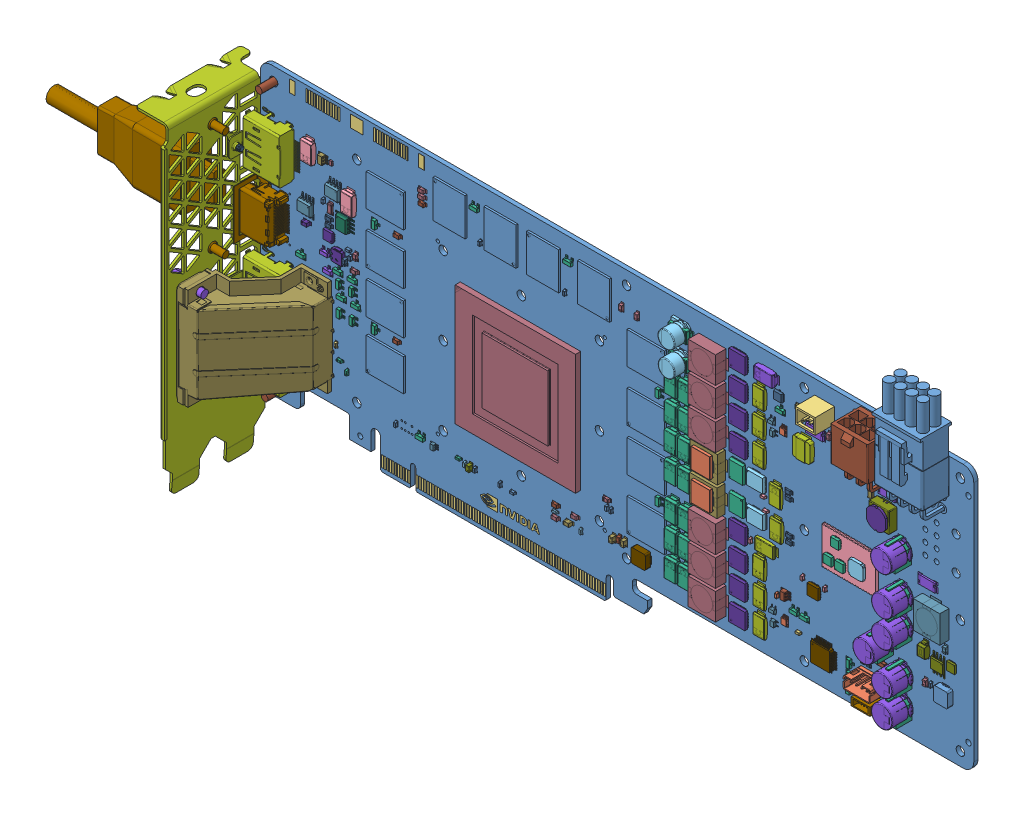
SolidWorks assembly PG600 SKU 0 3D Model, configuration Default. Lengths in mm.
Overall size (340.29 147.26 41.89).
548 component instances, 102 part files, 0 mates.
Components (placement in the parent):
- 142-1G600-1000-A05-1: 142-1G600-1000-A05 [Default] at origin size (266.7 111.15 1.57)
- 085-0009-000_1-1: 085-0009-000_1 [Default] at (20.943 18.972 0) x (1 0 0) z (0 0 -1) size (4.7 8 1.1)
- 075-0186-000_1-1: 075-0186-000_1 [Default] at (174.857 94.825 1.575) x (-1 0 0) z (0 0 1) size (7.4 5.75 10.67)
- 092-0023-000_1-1: 092-0023-000_1 [Default] at (-32.5 68.3 1.575) x (-1 0 0) z (0 0 1) size (3.05 1.35 0.81)
- 041-0139-000_1-1: 041-0139-000_1 [Default] at (120.487 94.534 1.575) x (-1 0 0) z (0 0 1) size (8.76 6.6 6.13)
- 041-0139-000_1-2: 041-0139-000_1 [Default] at (120.582 85.179 1.575) x (-1 0 0) z (0 0 1) size (8.76 6.6 6.13)
- CAP_SMD_066X066_B_6000_GREY-1: CAP_SMD_066X066_B_6000_GREY [Default] at (195.893 32.152 1.575) x (0 -1 0) z (0 0 1) size (8.76 6.8 6)
- CAP_SMD_066X066_B_6000_GREY-2: CAP_SMD_066X066_B_6000_GREY [Default] at (202.884 24.662 1.575) x (0 -1 0) z (0 0 1) size (8.76 6.8 6)
- CAP_SMD_066X066_B_6000_GREY-3: CAP_SMD_066X066_B_6000_GREY [Default] at (202.882 14.586 1.575) x (0 -1 0) z (0 0 1) size (8.76 6.8 6)
- CAP_SMD_066X066_B_6000_GREY-4: CAP_SMD_066X066_B_6000_GREY [Default] at (202.893 40.377 1.575) x (0 -1 0) z (0 0 1) size (8.76 6.8 6)
- CAP_SMD_066X066_B_6000_GREY-5: CAP_SMD_066X066_B_6000_GREY [Default] at (202.941 50.414 1.575) x (0 -1 0) z (0 0 1) size (8.76 6.8 6)
- CAP_SMD_066X066_B_6000_GREY-6: CAP_SMD_066X066_B_6000_GREY [Default] at (202.578 64.708 1.575) x (0 -1 0) z (0 0 1) size (8.76 6.8 6)
- 080-1128-000_3-1: 080-1128-000_3 [Default] at (-34.025 79.504 1.575) size (15.59 18.32 13.18)
- 080-1128-000_3-2: 080-1128-000_3 [Default] at (-34.025 11.683 1.575) size (15.59 18.32 13.18)
- 080-1128-000_3-3: 080-1128-000_3 [Default] at (-34.025 34.29 1.575) size (15.59 18.32 13.18)
- 032-0286-000_1-1: 032-0286-000_1 [Default] at (195.95 32.23 1.575) x (0 1 0) z (0 0 1) size (8 8 10.56)
- 032-0286-000_1-2: 032-0286-000_1 [Default] at (202.578 64.708 1.575) x (0 1 0) z (0 0 1) size (8 8 10.56)
- 032-0286-000_1-3: 032-0286-000_1 [Default] at (202.884 24.662 1.575) x (0 1 0) z (0 0 1) size (8 8 10.56)
- 032-0286-000_1-4: 032-0286-000_1 [Default] at (202.882 14.586 1.575) x (0 1 0) z (0 0 1) size (8 8 10.56)
- 032-0286-000_1-5: 032-0286-000_1 [Default] at (202.893 40.377 1.575) x (0 1 0) z (0 0 1) size (8 8 10.56)
- 032-0286-000_1-6: 032-0286-000_1 [Default] at (202.941 50.414 1.575) x (0 1 0) z (0 0 1) size (8 8 10.56)
- 065-0573-000_3-1: 065-0573-000_3 [Default] at (191.77 10.711 1.575) size (7.8 4.2 4.7)
- 195-2659-000_1-1: 195-2659-000_1 [Default] at (-11.4 64.9 1.575) x (-1 0 0) z (0 0 1) size (3.05 1.27 0.65)
- 195-2659-000_1-2: 195-2659-000_1 [Default] at (-11.4 62.7 1.575) x (-1 0 0) z (0 0 1) size (3.05 1.27 0.65)
- 039-0122-000_1-1: 039-0122-000_1 [Default] at (35.525 33.7 0) x (1 0 0) z (0 0 -1) size (3.05 1.27 0.95)
- 039-0122-000_1-2: 039-0122-000_1 [Default] at (72.9 71.075 0) x (0 -1 0) z (0 0 -1) size (3.05 1.27 0.95)
- 039-0127-000_1-1: 039-0127-000_1 [Default] at (55.7 37.85 0) x (1 0 0) z (0 0 -1) size (3.05 1.27 1.5)
- 039-0123-000_1-1: 039-0123-000_1 [Default] at (-2.83 51.24 0) x (0 -1 0) z (0 0 -1) size (3.05 1.27 0.95)
- 039-0123-000_1-2: 039-0123-000_1 [Default] at (10.45 18.82 0) x (1 0 0) z (0 0 -1) size (3.05 1.27 0.95)
- 039-0123-000_1-3: 039-0123-000_1 [Default] at (-0.72 49.54 0) x (0 -1 0) z (0 0 -1) size (3.05 1.27 0.95)
- 039-0123-000_1-4: 039-0123-000_1 [Default] at (-1.775 55.408 0) x (0 -1 0) z (0 0 -1) size (3.05 1.27 0.95)
- 039-0123-000_1-5: 039-0123-000_1 [Default] at (-1.76 64.49 0) x (0 -1 0) z (0 0 -1) size (3.05 1.27 0.95)
- 039-0123-000_1-6: 039-0123-000_1 [Default] at (-1.9 76.4 0) x (0 -1 0) z (0 0 -1) size (3.05 1.27 0.95)
- 039-0123-000_1-7: 039-0123-000_1 [Default] at (-2 83.1 0) x (0 -1 0) z (0 0 -1) size (3.05 1.27 0.95)
- 039-0123-000_1-8: 039-0123-000_1 [Default] at (22.11 26.9 0) x (1 0 0) z (0 0 -1) size (3.05 1.27 0.95)
- 195-2659-000_1-3: 195-2659-000_1 [Default] at (188.38 21.821 1.575) x (0 -1 0) z (0 0 1) size (3.05 1.27 0.65)
- 195-2659-000_1-4: 195-2659-000_1 [Default] at (190.5 21.844 1.575) x (0 -1 0) z (0 0 1) size (3.05 1.27 0.65)
- 039-0122-000_1-3: 039-0122-000_1 [Default] at (-20.619 61.841 0) x (1 0 0) z (0 0 -1) size (3.05 1.27 0.95)
- 039-0183-000_1-1: 039-0183-000_1 [Default] at (172.15 38.75 0) x (0 1 0) z (0 0 -1) size (3.05 1.27 0.95)
- 039-0123-000_1-9: 039-0123-000_1 [Default] at (-10.025 67.525 0) x (-1 0 0) z (0 0 -1) size (3.05 1.27 0.95)
- 039-0123-000_1-10: 039-0123-000_1 [Default] at (175.7 88 1.575) x (0 1 0) z (0 0 1) size (3.05 1.27 0.95)
- 039-0123-000_1-11: 039-0123-000_1 [Default] at (180.3 85.6 1.575) x (-1 0 0) z (0 0 1) size (3.05 1.27 0.95)
- 039-0123-000_1-12: 039-0123-000_1 [Default] at (184.3 88.7 1.575) x (0 -1 0) z (0 0 1) size (3.05 1.27 0.95)
- 195-1593-000_1-1: 195-1593-000_1 [Default] at (162.725 84.45 0) x (1 0 0) z (0 0 -1) size (3.05 1.27 0.7)
- 195-1593-000_1-2: 195-1593-000_1 [Default] at (162.75 82.3 0) x (1 0 0) z (0 0 -1) size (3.05 1.27 0.7)
- 039-0123-000_1-13: 039-0123-000_1 [Default] at (6.35 17.11 0) x (-1 0 0) z (0 0 -1) size (3.05 1.27 0.95)
- 039-0123-000_1-14: 039-0123-000_1 [Default] at (-1.3 57.63 1.575) x (0 -1 0) z (0 0 1) size (3.05 1.27 0.95)
- 039-0123-000_1-15: 039-0123-000_1 [Default] at (-1.855 72.5 0) x (0 -1 0) z (0 0 -1) size (3.05 1.27 0.95)
- 039-0123-000_1-16: 039-0123-000_1 [Default] at (-1.725 52.725 1.575) size (3.05 1.27 0.95)
- 039-0123-000_1-17: 039-0123-000_1 [Default] at (83.95 31.45 0) x (0 1 0) z (0 0 -1) size (3.05 1.27 0.95)
- 039-0123-000_1-18: 039-0123-000_1 [Default] at (80.65 14.5 1.575) x (-1 0 0) z (0 0 1) size (3.05 1.27 0.95)
- 039-0123-000_1-19: 039-0123-000_1 [Default] at (73.405 10.52 1.575) x (-1 0 0) z (0 0 1) size (3.05 1.27 0.95)
- 039-0123-000_1-20: 039-0123-000_1 [Default] at (86.1 31.8 0) x (0 1 0) z (0 0 -1) size (3.05 1.27 0.95)
- 039-0123-000_1-21: 039-0123-000_1 [Default] at (211.708 26.314 1.575) x (0 1 0) z (0 0 1) size (3.05 1.27 0.95)
- 039-0149-000_1-1: 039-0149-000_1 [Default] at (41.5 10.9 1.575) x (0 -1 0) z (0 0 1) size (3.05 1.27 1.45)
- 039-0122-000_1-4: 039-0122-000_1 [Default] at (96.025 17.979 0) x (0 1 0) z (0 0 -1) size (3.05 1.27 0.95)
- 039-0122-000_1-5: 039-0122-000_1 [Default] at (73.428 14.643 1.575) x (-1 0 0) z (0 0 1) size (3.05 1.27 0.95)
- 039-0123-000_1-22: 039-0123-000_1 [Default] at (35.525 42.275 0) x (1 0 0) z (0 0 -1) size (3.05 1.27 0.95)
- 039-0123-000_1-23: 039-0123-000_1 [Default] at (49.833 47.9 0) x (1 0 0) z (0 0 -1) size (3.05 1.27 0.95)
- 039-0122-000_1-6: 039-0122-000_1 [Default] at (35.525 59.075 0) x (1 0 0) z (0 0 -1) size (3.05 1.27 0.95)
- 039-0127-000_1-2: 039-0127-000_1 [Default] at (78.45 11.45 1.575) x (-1 0 0) z (0 0 1) size (3.05 1.27 1.5)
- 039-0122-000_1-7: 039-0122-000_1 [Default] at (97.194 15.396 1.575) x (0 -1 0) z (0 0 1) size (3.05 1.27 0.95)
- 039-0123-000_1-24: 039-0123-000_1 [Default] at (98.646 15.219 0) x (-1 0 0) z (0 0 -1) size (3.05 1.27 0.95)
- 039-0123-000_1-25: 039-0123-000_1 [Default] at (69.8 34.95 0) x (0 1 0) z (0 0 -1) size (3.05 1.27 0.95)
- 039-0123-000_1-26: 039-0123-000_1 [Default] at (92.545 26 1.575) size (3.05 1.27 0.95)
- 039-0123-000_1-27: 039-0123-000_1 [Default] at (103.581 14.199 0) x (0 -1 0) z (0 0 -1) size (3.05 1.27 0.95)
- 039-0127-000_1-3: 039-0127-000_1 [Default] at (95.03 14.63 1.575) x (0 -1 0) z (0 0 1) size (3.05 1.27 1.5)
- 039-0127-000_1-4: 039-0127-000_1 [Default] at (99.35 15.506 1.575) x (0 -1 0) z (0 0 1) size (3.05 1.27 1.5)
- 039-0123-000_1-28: 039-0123-000_1 [Default] at (95.803 14.546 0) x (0 1 0) z (0 0 -1) size (3.05 1.27 0.95)
- 039-0127-000_1-5: 039-0127-000_1 [Default] at (52.698 38.9 0) x (0 -1 0) z (0 0 -1) size (3.05 1.27 1.5)
- 039-0127-000_1-6: 039-0127-000_1 [Default] at (67.63 38.9 0) x (0 -1 0) z (0 0 -1) size (3.05 1.27 1.5)
- 039-0127-000_1-7: 039-0127-000_1 [Default] at (55.7 39.955 0) x (-1 0 0) z (0 0 -1) size (3.05 1.27 1.5)
- 039-0127-000_1-8: 039-0127-000_1 [Default] at (64.677 39.955 0) x (1 0 0) z (0 0 -1) size (3.05 1.27 1.5)
- 039-0127-000_1-9: 039-0127-000_1 [Default] at (64.673 37.85 0) x (-1 0 0) z (0 0 -1) size (3.05 1.27 1.5)
- 039-0127-000_1-10: 039-0127-000_1 [Default] at (59.55 50.825 0) x (1 0 0) z (0 0 -1) size (3.05 1.27 1.5)
- 039-0127-000_1-11: 039-0127-000_1 [Default] at (59.55 52.95 0) x (-1 0 0) z (0 0 -1) size (3.05 1.27 1.5)
- 039-0127-000_1-12: 039-0127-000_1 [Default] at (58.745 55.905 0) x (0 -1 0) z (0 0 -1) size (3.05 1.27 1.5)
- 039-0127-000_1-13: 039-0127-000_1 [Default] at (70.425 47.9 0) x (-1 0 0) z (0 0 -1) size (3.05 1.27 1.5)
- 039-0127-000_1-14: 039-0127-000_1 [Default] at (70.425 54 0) x (-1 0 0) z (0 0 -1) size (3.05 1.27 1.5)
- 039-0123-000_1-29: 039-0123-000_1 [Default] at (84.925 50.525 0) x (-1 0 0) z (0 0 -1) size (3.05 1.27 0.95)
- 039-0123-000_1-30: 039-0123-000_1 [Default] at (47.5 71.075 0) x (0 -1 0) z (0 0 -1) size (3.05 1.27 0.95)
- 039-0123-000_1-31: 039-0123-000_1 [Default] at (61.695 56.125 0) x (0 -1 0) z (0 0 -1) size (3.05 1.27 0.95)
- 039-0123-000_1-32: 039-0123-000_1 [Default] at (84.2 34.825 0) x (0 -1 0) z (0 0 -1) size (3.05 1.27 0.95)
- 039-0123-000_1-33: 039-0123-000_1 [Default] at (-25.756 82.681 0) x (-1 0 0) z (0 0 -1) size (3.05 1.27 0.95)
- 039-0183-000_1-2: 039-0183-000_1 [Default] at (219.175 40.665 1.575) x (0 1 0) z (0 0 1) size (3.05 1.27 0.95)
- 195-2659-000_1-5: 195-2659-000_1 [Default] at (156.375 93.375 0) x (-1 0 0) z (0 0 -1) size (3.05 1.27 0.65)
- 039-0123-000_1-34: 039-0123-000_1 [Default] at (113.785 14.62 0) x (0 1 0) z (0 0 -1) size (3.05 1.27 0.95)
- 039-0123-000_1-35: 039-0123-000_1 [Default] at (24.275 48.025 0) x (-1 0 0) z (0 0 -1) size (3.05 1.27 0.95)
- 039-0123-000_1-36: 039-0123-000_1 [Default] at (24.225 45.55 0) x (-1 0 0) z (0 0 -1) size (3.05 1.27 0.95)
- 039-0123-000_1-37: 039-0123-000_1 [Default] at (118.603 81.12 0) x (0 1 0) z (0 0 -1) size (3.05 1.27 0.95)
- 039-0123-000_1-38: 039-0123-000_1 [Default] at (118.603 73.283 0) x (0 1 0) z (0 0 -1) size (3.05 1.27 0.95)
- 039-0123-000_1-39: 039-0123-000_1 [Default] at (118.603 66.408 0) x (0 1 0) z (0 0 -1) size (3.05 1.27 0.95)
- 039-0123-000_1-40: 039-0123-000_1 [Default] at (120.142 63.5 0) x (-1 0 0) z (0 0 -1) size (3.05 1.27 0.95)
- 039-0123-000_1-41: 039-0123-000_1 [Default] at (118.7 49.1 0) x (0 -1 0) z (0 0 -1) size (3.05 1.27 0.95)
- 039-0123-000_1-42: 039-0123-000_1 [Default] at (118.603 38.283 0) x (0 1 0) z (0 0 -1) size (3.05 1.27 0.95)
- 039-0123-000_1-43: 039-0123-000_1 [Default] at (118.603 31.408 0) x (0 1 0) z (0 0 -1) size (3.05 1.27 0.95)
- 039-0123-000_1-44: 039-0123-000_1 [Default] at (118.603 21.008 0) x (0 -1 0) z (0 0 -1) size (3.05 1.27 0.95)
- 039-0123-000_1-45: 039-0123-000_1 [Default] at (114 89.35 0) x (1 0 0) z (0 0 -1) size (3.05 1.27 0.95)
- 039-0123-000_1-46: 039-0123-000_1 [Default] at (103.9 90.95 0) x (0 -1 0) z (0 0 -1) size (3.05 1.27 0.95)
- 039-0123-000_1-47: 039-0123-000_1 [Default] at (103.9 90.95 1.575) x (0 -1 0) z (0 0 1) size (3.05 1.27 0.95)
- 039-0123-000_1-48: 039-0123-000_1 [Default] at (98.101 90.925 1.575) x (0 -1 0) z (0 0 1) size (3.05 1.27 0.95)
- 039-0122-000_1-8: 039-0122-000_1 [Default] at (14 37.95 1.575) x (-1 0 0) z (0 0 1) size (3.05 1.27 0.95)
- 039-0123-000_1-49: 039-0123-000_1 [Default] at (23.428 91.558 1.575) x (-1 0 0) z (0 0 1) size (3.05 1.27 0.95)
- 039-0123-000_1-50: 039-0123-000_1 [Default] at (23.5 89.1 0) x (-1 0 0) z (0 0 -1) size (3.05 1.27 0.95)
- 039-0122-000_1-9: 039-0122-000_1 [Default] at (23.546 87.229 1.575) x (-1 0 0) z (0 0 1) size (3.05 1.27 0.95)
- 039-0123-000_1-51: 039-0123-000_1 [Default] at (23.428 89.433 1.575) x (-1 0 0) z (0 0 1) size (3.05 1.27 0.95)
- 039-0123-000_1-52: 039-0123-000_1 [Default] at (21.8 85.9 0) x (1 0 0) z (0 0 -1) size (3.05 1.27 0.95)
- 039-0122-000_1-10: 039-0122-000_1 [Default] at (14.275 72.275 1.575) x (-1 0 0) z (0 0 1) size (3.05 1.27 0.95)
- 039-0183-000_1-3: 039-0183-000_1 [Default] at (150.05 23.325 1.575) x (0 1 0) z (0 0 1) size (3.05 1.27 0.95)
- 039-0183-000_1-4: 039-0183-000_1 [Default] at (150 32.875 1.575) x (0 1 0) z (0 0 1) size (3.05 1.27 0.95)
- 039-0183-000_1-5: 039-0183-000_1 [Default] at (148.667 70.869 0) x (-1 0 0) z (0 0 -1) size (3.05 1.27 0.95)
- 039-0183-000_1-6: 039-0183-000_1 [Default] at (148.66 87.864 0) x (0 1 0) z (0 0 -1) size (3.05 1.27 0.95)
- 039-0183-000_1-7: 039-0183-000_1 [Default] at (149.052 17.91 0) x (0 -1 0) z (0 0 -1) size (3.05 1.27 0.95)
- 039-0183-000_1-8: 039-0183-000_1 [Default] at (157.626 48.088 1.575) x (0 1 0) z (0 0 1) size (3.05 1.27 0.95)
- 039-0183-000_1-9: 039-0183-000_1 [Default] at (155.25 48.082 1.575) x (0 1 0) z (0 0 1) size (3.05 1.27 0.95)
- 039-0183-000_1-10: 039-0183-000_1 [Default] at (154.836 59.015 1.575) x (0 -1 0) z (0 0 1) size (3.05 1.27 0.95)
- 039-0183-000_1-11: 039-0183-000_1 [Default] at (157.186 59.015 1.575) x (0 -1 0) z (0 0 1) size (3.05 1.27 0.95)
- 039-0183-000_1-12: 039-0183-000_1 [Default] at (149.889 87.904 1.575) x (0 1 0) z (0 0 1) size (3.05 1.27 0.95)
- 039-0183-000_1-13: 039-0183-000_1 [Default] at (152.248 9.523 0) x (1 0 0) z (0 0 -1) size (3.05 1.27 0.95)
- 039-0183-000_1-14: 039-0183-000_1 [Default] at (149.392 35.661 0) x (0 -1 0) z (0 0 -1) size (3.05 1.27 0.95)
- 039-0183-000_1-15: 039-0183-000_1 [Default] at (152.456 96.335 1.575) size (3.05 1.27 0.95)
- 039-0183-000_1-16: 039-0183-000_1 [Default] at (152.075 40.3 1.575) size (3.05 1.27 0.95)
- 039-0183-000_1-17: 039-0183-000_1 [Default] at (149.849 78.501 1.575) x (0 1 0) z (0 0 1) size (3.05 1.27 0.95)
- 039-0183-000_1-18: 039-0183-000_1 [Default] at (148.59 96.901 0) x (0 1 0) z (0 0 -1) size (3.05 1.27 0.95)
- 039-0183-000_1-19: 039-0183-000_1 [Default] at (150.075 13.925 1.575) x (0 1 0) z (0 0 1) size (3.05 1.27 0.95)
- 039-0183-000_1-20: 039-0183-000_1 [Default] at (149.028 26.771 0) x (0 -1 0) z (0 0 -1) size (3.05 1.27 0.95)
- 039-0183-000_1-21: 039-0183-000_1 [Default] at (149.86 69.061 1.575) x (0 1 0) z (0 0 1) size (3.05 1.27 0.95)
- 039-0183-000_1-22: 039-0183-000_1 [Default] at (148.027 77.993 0) x (0 1 0) z (0 0 -1) size (3.05 1.27 0.95)
- 039-0123-000_1-53: 039-0123-000_1 [Default] at (-27.475 15.45 0) x (-1 0 0) z (0 0 -1) size (3.05 1.27 0.95)
- 039-0128-000_1-1: 039-0128-000_1 [Default] at (-19.638 59.56 1.575) x (-1 0 0) z (0 0 1) size (3.05 1.27 1.45)
- 039-0123-000_1-54: 039-0123-000_1 [Default] at (-28.04 36.25 0) x (1 0 0) z (0 0 -1) size (3.05 1.27 0.95)
- 039-0186-000_1-1: 039-0186-000_1 [Default] at (196.42 58.81 0) x (0 1 0) z (0 0 -1) size (3.05 1.27 0.85)
- 039-0186-000_1-2: 039-0186-000_1 [Default] at (204.6 58.55 0) x (0 1 0) z (0 0 -1) size (3.05 1.27 0.85)
- 195-2659-000_1-6: 195-2659-000_1 [Default] at (160.434 60.221 1.575) x (-1 0 0) z (0 0 1) size (3.05 1.27 0.65)
- 195-2659-000_1-7: 195-2659-000_1 [Default] at (160.413 62.392 1.575) x (-1 0 0) z (0 0 1) size (3.05 1.27 0.65)
- 195-2659-000_1-8: 195-2659-000_1 [Default] at (160.709 48.299 1.575) size (3.05 1.27 0.65)
- 195-2659-000_1-9: 195-2659-000_1 [Default] at (160.73 46.117 1.575) size (3.05 1.27 0.65)
- 130-0445-000_2-1: 130-0445-000_2 [Default] at (131.45 47.9 1.575) x (-1 0 0) z (0 0 1) size (8.4 6.73 3.02)
- 130-0445-000_2-2: 130-0445-000_2 [Default] at (131.509 58.802 1.575) x (-1 0 0) z (0 0 1) size (8.4 6.73 3.02)
- 115-1357-000_2-1: 115-1357-000_2 [Default] at (158.697 81.194 1.575) x (-1 0 0) z (0 0 1) size (2.04 3.61 0.94)
- 115-1357-000_2-2: 115-1357-000_2 [Default] at (159.182 19.863 1.575) x (-1 0 0) z (0 0 1) size (2.04 3.61 0.94)
- 065-0301-000_1-1: 065-0301-000_1 [Default] at (0 0 1.575) size (50.45 4.5 0.04)
- 041-0188-000_1-1: 041-0188-000_1 [Default] at (-18.6 83.4 1.575) x (0 1 0) z (0 0 1) size (8.64 4.39 1.93)
- 041-0188-000_1-2: 041-0188-000_1 [Default] at (-3.42 74.173 1.575) x (0 1 0) z (0 0 1) size (8.64 4.39 1.93)
- 041-0190-000_2-1: 041-0190-000_2 [Default] at (134.727 44.853 0) x (1 0 0) z (0 0 -1) size (8.64 4.39 1.55)
- 041-0085-000_2-1: 041-0085-000_2 [Default] at (120.582 94.59 1.575) x (-1 0 0) z (0 0 1) size (8.64 4.39 2.14)
- 041-0085-000_2-2: 041-0085-000_2 [Default] at (120.582 85.179 1.575) x (-1 0 0) z (0 0 1) size (8.64 4.39 2.14)
- 032-0070-000_1-1: 032-0070-000_1 [Default] at (156.036 59.04 1.575) x (0 -1 0) z (0 0 1) size (8.64 4.4 1.24)
- 032-0070-000_1-2: 032-0070-000_1 [Default] at (156.301 48.063 1.575) x (0 1 0) z (0 0 1) size (8.64 4.4 1.24)
- 032-0070-000_1-3: 032-0070-000_1 [Default] at (149.889 87.904 1.575) x (0 1 0) z (0 0 1) size (8.64 4.4 1.24)
- 032-0070-000_1-4: 032-0070-000_1 [Default] at (149.849 78.501 1.575) x (0 1 0) z (0 0 1) size (8.64 4.4 1.24)
- 032-0070-000_1-5: 032-0070-000_1 [Default] at (149.86 69.061 1.575) x (0 1 0) z (0 0 1) size (8.64 4.4 1.24)
- 032-0070-000_1-6: 032-0070-000_1 [Default] at (150 32.875 1.575) x (0 1 0) z (0 0 1) size (8.64 4.4 1.24)
- 032-0070-000_1-7: 032-0070-000_1 [Default] at (150.075 13.925 1.575) x (0 1 0) z (0 0 1) size (8.64 4.4 1.24)
- 032-0070-000_1-8: 032-0070-000_1 [Default] at (150.05 23.325 1.575) x (0 1 0) z (0 0 1) size (8.64 4.4 1.24)
- 041-0196-000_1-1: 041-0196-000_1 [Default] at (152.456 96.335 1.575) size (8.64 4.39 2.04)
- 032-0070-000_1-9: 032-0070-000_1 [Default] at (152.075 40.3 1.575) size (8.64 4.4 1.24)
- 041-0085-000_2-3: 041-0085-000_2 [Default] at (122.878 16.429 1.575) x (0 -1 0) z (0 0 1) size (8.64 4.39 2.14)
- 041-0085-000_2-4: 041-0085-000_2 [Default] at (122.878 25.902 1.575) x (0 1 0) z (0 0 1) size (8.64 4.39 2.14)
- 041-0085-000_2-5: 041-0085-000_2 [Default] at (122.808 47.973 1.575) x (0 -1 0) z (0 0 1) size (8.64 4.39 2.14)
- 041-0085-000_2-6: 041-0085-000_2 [Default] at (122.808 57.645 1.575) x (0 1 0) z (0 0 1) size (8.64 4.39 2.14)
- 041-0196-000_1-2: 041-0196-000_1 [Default] at (202.941 50.414 1.575) x (0 -1 0) z (0 0 1) size (8.64 4.39 2.04)
- 041-0085-000_2-7: 041-0085-000_2 [Default] at (117.82 16.379 1.575) x (0 -1 0) z (0 0 1) size (8.64 4.39 2.14)
- 041-0085-000_2-8: 041-0085-000_2 [Default] at (117.82 25.902 1.575) x (0 1 0) z (0 0 1) size (8.64 4.39 2.14)
- 041-0085-000_2-9: 041-0085-000_2 [Default] at (122.878 35.327 1.575) x (0 -1 0) z (0 0 1) size (8.64 4.39 2.14)
- 041-0196-000_1-3: 041-0196-000_1 [Default] at (195.95 32.48 1.575) x (0 -1 0) z (0 0 1) size (8.64 4.39 2.04)
- 041-0196-000_1-4: 041-0196-000_1 [Default] at (202.884 24.662 1.575) x (0 -1 0) z (0 0 1) size (8.64 4.39 2.04)
- 041-0196-000_1-5: 041-0196-000_1 [Default] at (202.882 14.586 1.575) x (0 -1 0) z (0 0 1) size (8.64 4.39 2.04)
- 041-0196-000_1-6: 041-0196-000_1 [Default] at (202.893 40.377 1.575) x (0 -1 0) z (0 0 1) size (8.64 4.39 2.04)
- 041-0196-000_1-7: 041-0196-000_1 [Default] at (202.578 64.708 1.575) x (0 -1 0) z (0 0 1) size (8.64 4.39 2.04)
- 041-0085-000_2-10: 041-0085-000_2 [Default] at (117.76 57.691 1.575) x (0 1 0) z (0 0 1) size (8.64 4.39 2.14)
- 041-0085-000_2-11: 041-0085-000_2 [Default] at (117.76 47.973 1.575) x (0 -1 0) z (0 0 1) size (8.64 4.39 2.14)
- 041-0085-000_2-12: 041-0085-000_2 [Default] at (122.878 76.335 1.575) x (0 -1 0) z (0 0 1) size (8.64 4.39 2.14)
- 041-0085-000_2-13: 041-0085-000_2 [Default] at (117.82 76.335 1.575) x (0 -1 0) z (0 0 1) size (8.64 4.39 2.14)
- 041-0085-000_2-14: 041-0085-000_2 [Default] at (122.878 66.927 1.575) x (0 1 0) z (0 0 1) size (8.64 4.39 2.14)
- 041-0085-000_2-15: 041-0085-000_2 [Default] at (117.82 66.927 1.575) x (0 1 0) z (0 0 1) size (8.64 4.39 2.14)
- 041-0190-000_2-2: 041-0190-000_2 [Default] at (133.35 22.479 0) x (1 0 0) z (0 0 -1) size (8.64 4.39 1.55)
- 041-0085-000_2-16: 041-0085-000_2 [Default] at (117.82 35.352 1.575) x (0 -1 0) z (0 0 1) size (8.64 4.39 2.14)
- 041-0190-000_2-3: 041-0190-000_2 [Default] at (133.35 77.978 0) x (1 0 0) z (0 0 -1) size (8.64 4.39 1.55)
- 032-0299-000_1-1: 032-0299-000_1 [Default] at (60.2 41.4 0) x (0 1 0) z (0 0 -1) size (8.64 4.39 1.55)
- 032-0299-000_1-2: 032-0299-000_1 [Default] at (54.185 50.187 0) x (0 -1 0) z (0 0 -1) size (8.64 4.39 1.55)
- 032-0299-000_1-3: 032-0299-000_1 [Default] at (66.215 50.187 0) x (0 -1 0) z (0 0 -1) size (8.64 4.39 1.55)
- 100-0028-000_1-1: 100-0028-000_1 [Default] at (-9.625 54.35 1.575) x (0 1 0) z (0 0 1) size (3.05 1.27 1.22)
- 100-0028-000_1-2: 100-0028-000_1 [Default] at (-7.4 54.65 1.575) x (0 1 0) z (0 0 1) size (3.05 1.27 1.22)
- 100-0028-000_1-3: 100-0028-000_1 [Default] at (-5.175 54.2 1.575) x (0 1 0) z (0 0 1) size (3.05 1.27 1.22)
- 315-0756-000_1-1: 315-0756-000_1 [Default] at (159.23 28.51 1.575) x (0 1 0) z (0 0 1) size (2.9 3.58 1.45)
- 115-0121-000_1-1: 115-0121-000_1 [Default] at (-13.747 83.189 1.575) x (0 1 0) z (0 0 1) size (2.9 3.58 1.45)
- 115-0398-000_1-1: 115-0398-000_1 [Default] at (-10.55 83.34 1.575) size (1.16 1.5 0.56)
- 300-0766-000_1-1: 300-0766-000_1 [Default] at (204.857 70.96 0) x (0 -1 0) z (0 0 -1) size (2.1 2.4 0.86)
- 316-0134-000_3-1: 316-0134-000_3 [Default] at (108.01 13.735 0) x (0 -1 0) z (0 0 -1) size (3 3.5 0.8)
- 315-0829-000_4-1: 315-0829-000_4 [Default] at (221.45 36.11 1.575) x (-1 0 0) z (0 0 1) size (3 3.5 0.8)
- 305-0092-000_1-1: 305-0092-000_1 [Default] at (-11.3 59.5 1.575) x (-1 0 0) z (0 0 1) size (3.81 3.5 0.91)
- 115-1286-000_2-1: 115-1286-000_2 [Default] at (173.55 16.15 1.575) size (9.65 9.65 1.6)
- 161-0163-100_1-1: 161-0163-100_1 [Default] at (10.2 62.775 1.575) x (0 1 0) z (0 0 1) size (12 14 0.75)
- 161-0163-100_1-2: 161-0163-100_1 [Default] at (10.2 62.775 0) x (0 1 0) z (0 0 -1) size (12 14 0.75)
- 161-0163-100_1-3: 161-0163-100_1 [Default] at (10.2 81.775 1.575) x (0 -1 0) z (0 0 1) size (12 14 0.75)
- 161-0163-100_1-4: 161-0163-100_1 [Default] at (10.2 81.775 0) x (0 -1 0) z (0 0 -1) size (12 14 0.75)
- 161-0163-100_1-5: 161-0163-100_1 [Default] at (34.2 91.4 1.575) size (12 14 0.75)
- 161-0163-100_1-6: 161-0163-100_1 [Default] at (34.2 91.4 0) x (1 0 0) z (0 0 -1) size (12 14 0.75)
- 161-0163-100_1-7: 161-0163-100_1 [Default] at (10.2 46.8 1.575) x (0 -1 0) z (0 0 1) size (12 14 0.75)
- 161-0163-100_1-8: 161-0163-100_1 [Default] at (10.2 46.8 0) x (0 -1 0) z (0 0 -1) size (12 14 0.75)
- 161-0163-100_1-9: 161-0163-100_1 [Default] at (10.2 28.75 1.575) x (0 1 0) z (0 0 1) size (12 14 0.75)
- 161-0163-100_1-10: 161-0163-100_1 [Default] at (10.2 28.75 0) x (0 1 0) z (0 0 -1) size (12 14 0.75)
- 161-0163-100_1-11: 161-0163-100_1 [Default] at (53.2 91.4 1.575) x (-1 0 0) z (0 0 1) size (12 14 0.75)
- 161-0163-100_1-12: 161-0163-100_1 [Default] at (53.2 91.4 0) x (-1 0 0) z (0 0 -1) size (12 14 0.75)
- 161-0163-100_1-13: 161-0163-100_1 [Default] at (69.2 91.4 1.575) size (12 14 0.75)
- 161-0163-100_1-14: 161-0163-100_1 [Default] at (69.2 91.4 0) x (1 0 0) z (0 0 -1) size (12 14 0.75)
- 161-0163-100_1-15: 161-0163-100_1 [Default] at (88.2 91.4 1.575) x (-1 0 0) z (0 0 1) size (12 14 0.75)
- 161-0163-100_1-16: 161-0163-100_1 [Default] at (88.2 91.4 0) x (-1 0 0) z (0 0 -1) size (12 14 0.75)
- 161-0163-100_1-17: 161-0163-100_1 [Default] at (107.7 79.4 1.575) x (0 -1 0) z (0 0 1) size (12 14 0.75)
- 161-0163-100_1-18: 161-0163-100_1 [Default] at (107.7 79.4 0) x (0 -1 0) z (0 0 -1) size (12 14 0.75)
- 161-0163-100_1-19: 161-0163-100_1 [Default] at (107.7 60.4 1.575) x (0 1 0) z (0 0 1) size (12 14 0.75)
- 161-0163-100_1-20: 161-0163-100_1 [Default] at (107.7 60.4 0) x (0 1 0) z (0 0 -1) size (12 14 0.75)
- 161-0163-100_1-21: 161-0163-100_1 [Default] at (107.7 44.4 1.575) x (0 -1 0) z (0 0 1) size (12 14 0.75)
- 161-0163-100_1-22: 161-0163-100_1 [Default] at (107.7 25.4 1.575) x (0 1 0) z (0 0 1) size (12 14 0.75)
- 161-0163-100_1-23: 161-0163-100_1 [Default] at (107.7 25.4 0) x (0 1 0) z (0 0 -1) size (12 14 0.75)
- 161-0163-100_1-24: 161-0163-100_1 [Default] at (107.7 44.4 0) x (0 -1 0) z (0 0 -1) size (12 14 0.75)
- 131-0786-000_1-1: 131-0786-000_1 [Default] at (131.236 58.867 1.575) x (-1 0 0) z (0 0 1) size (8.9 7.51 4.02)
- 131-0786-000_1-2: 131-0786-000_1 [Default] at (131.236 48.08 1.575) x (-1 0 0) z (0 0 1) size (8.9 7.51 4.02)
- 115-0732-000_1-1: 115-0732-000_1 [Default] at (134.75 35.075 0) x (1 0 0) z (0 0 -1) size (1.45 1.24 0.61)
- 115-0732-000_1-2: 115-0732-000_1 [Default] at (134.64 90.21 0) x (1 0 0) z (0 0 -1) size (1.45 1.24 0.61)
- 115-0967-000_1-1: 115-0967-000_1 [Default] at (159.192 19.829 1.575) x (-1 0 0) z (0 0 1) size (2 1.08 0.51)
- 115-0967-000_1-2: 115-0967-000_1 [Default] at (158.707 81.194 1.575) x (-1 0 0) z (0 0 1) size (2 1.08 0.51)
- 300-0250-000_1-1: 300-0250-000_1 [Default] at (148.55 48.207 1.575) x (0 -1 0) z (0 0 1) size (5.9 6.8 1.12)
- 300-0787-000_1-1: 300-0787-000_1 [Default] at (141.494 59.632 1.575) size (5.9 6.8 1.12)
- 300-0250-000_1-2: 300-0250-000_1 [Default] at (148.524 60.111 1.575) x (0 -1 0) z (0 0 1) size (5.9 6.8 1.12)
- 300-0787-000_1-2: 300-0787-000_1 [Default] at (141.494 48.886 1.575) x (-1 0 0) z (0 0 1) size (5.9 6.8 1.12)
- 131-0213-000_2-1: 131-0213-000_2 [Default] at (166.676 79.836 1.575) x (0 -1 0) z (0 0 1) size (8.13 6.48 2.16)
- 215-0139-000_2-1: 215-0139-000_2 [Default] at (170.37 86.796 1.575) size (7.39 3.64 0.64)
- 215-0139-000_2-2: 215-0139-000_2 [Default] at (212.36 58.765 1.575) size (7.39 3.64 0.64)
- 215-0139-000_2-3: 215-0139-000_2 [Default] at (197.434 80.578 1.575) size (7.39 3.64 0.64)
- 080-0424-000_1-1: 080-0424-000_1 [Default] at (-33 56.897 1.575) size (84.48 20.93 11.48)
- 300-0667-000_1-1: 300-0667-000_1 [Default] at (209.91 58.81 0) x (0 1 0) z (0 0 -1) size (3.6 3.75 0.91)
- 300-0667-000_1-2: 300-0667-000_1 [Default] at (201.12 58.849 0) x (0 1 0) z (0 0 -1) size (3.6 3.75 0.91)
- 300-0667-000_1-3: 300-0667-000_1 [Default] at (156.875 91.625 1.575) x (0 -1 0) z (0 0 1) size (3.6 3.75 0.91)
- 065-0415-000_2-1: 065-0415-000_2 [Default] at (190.19 89.67 1.575) size (14.2 19.73 16.66)
- 131-0560-000_2-1: 131-0560-000_2 [Default] at (131.463 58.875 1.575) x (0 1 0) z (0 0 1) size (9.91 11.94 3.03)
- 131-0560-000_2-2: 131-0560-000_2 [Default] at (131.336 47.953 1.575) x (0 1 0) z (0 0 1) size (9.91 11.94 3.03)
- 131-0397-000_2-1: 131-0397-000_2 [Default] at (131.763 91.799 1.575) x (0 1 0) z (0 0 1) size (9.91 11.94 4.02)
- 131-0397-000_2-2: 131-0397-000_2 [Default] at (131.764 80.889 1.575) x (0 1 0) z (0 0 1) size (9.91 11.94 4.02)
- 131-0397-000_2-3: 131-0397-000_2 [Default] at (131.764 69.978 1.575) x (0 1 0) z (0 0 1) size (9.91 11.94 4.02)
- 131-0397-000_2-4: 131-0397-000_2 [Default] at (131.764 36.993 1.575) x (0 1 0) z (0 0 1) size (9.91 11.94 4.02)
- 131-0397-000_2-5: 131-0397-000_2 [Default] at (131.764 26.083 1.575) x (0 1 0) z (0 0 1) size (9.91 11.94 4.02)
- 131-0397-000_2-6: 131-0397-000_2 [Default] at (131.764 15.173 1.575) x (0 1 0) z (0 0 1) size (9.91 11.94 4.02)
- 131-0134-000_3-1: 131-0134-000_3 [Default] at (215.26 49.24 1.575) x (-1 0 0) z (0 0 1) size (9.91 11.94 3.51)
- 131-0257-000_1-1: 131-0257-000_1 [Default] at (131.236 48.08 1.575) x (0 -1 0) z (0 0 1) size (6.81 7.48 3.08)
- 131-0257-000_1-2: 131-0257-000_1 [Default] at (131.236 58.867 1.575) x (0 -1 0) z (0 0 1) size (6.81 7.48 3.08)
- 090-0091-000_2-1: 090-0091-000_2 [Default] at (211.75 37.06 1.575) x (0 1 0) z (0 0 1) size (5.92 2.76 2.23)
- 131-0246-000_2-1: 131-0246-000_2 [Default] at (-7.625 54.65 1.575) x (0 1 0) z (0 0 1) size (4.96 4.06 1.22)
- 115-1066-000_2-1: 115-1066-000_2 [Default] at (180 90 1.575) x (-1 0 0) z (0 0 1) size (4.59 4.59 1.02)
- 039-0125-000_1-1: 039-0125-000_1 [Default] at (28.8 26.35 0) x (-1 0 0) z (0 0 -1) size (2 0.84 0.97)
- 039-0135-000_1-1: 039-0135-000_1 [Default] at (156.21 26.832 1.575) x (0 -1 0) z (0 0 1) size (2 0.84 0.97)
- 039-0037-000_1-1: 039-0037-000_1 [Default] at (164.3 18.8 1.575) x (-1 0 0) z (0 0 1) size (2 0.84 1.02)
- 039-0125-000_1-2: 039-0125-000_1 [Default] at (5.128 73.258 0) x (-1 0 0) z (0 0 -1) size (2 0.84 0.97)
- 039-0125-000_1-3: 039-0125-000_1 [Default] at (18.803 63.058 0) x (0 -1 0) z (0 0 -1) size (2 0.84 0.97)
- 039-0125-000_1-4: 039-0125-000_1 [Default] at (19.547 77.342 0) x (0 -1 0) z (0 0 -1) size (2 0.84 0.97)
- 039-0125-000_1-5: 039-0125-000_1 [Default] at (20.408 88.931 0) x (1 0 0) z (0 0 -1) size (2 0.84 0.97)
- 039-0125-000_1-6: 039-0125-000_1 [Default] at (24.9 85.6 0) x (-1 0 0) z (0 0 -1) size (2 0.84 0.97)
- 039-0125-000_1-7: 039-0125-000_1 [Default] at (24.9 87.2 0) x (-1 0 0) z (0 0 -1) size (2 0.84 0.97)
- 039-0125-000_1-8: 039-0125-000_1 [Default] at (29.403 82.508 0) x (-0.707107 -0.707107 0) z (0 0 -1) size (2 0.84 0.97)
- 039-0125-000_1-9: 039-0125-000_1 [Default] at (19.547 42.367 0) x (0 -1 0) z (0 0 -1) size (2 0.84 0.97)
- 039-0125-000_1-10: 039-0125-000_1 [Default] at (18.953 57.983 0) x (0 -1 0) z (0 0 -1) size (2 0.84 0.97)
- 039-0125-000_1-11: 039-0125-000_1 [Default] at (20.447 52.142 0) x (1 0 0) z (0 0 -1) size (2 0.84 0.97)
- 039-0125-000_1-12: 039-0125-000_1 [Default] at (18.803 29.033 0) x (0 -1 0) z (0 0 -1) size (2 0.84 0.97)
- 039-0125-000_1-13: 039-0125-000_1 [Default] at (19.1 34.5 0) x (0 -1 0) z (0 0 -1) size (2 0.84 0.97)
- 039-0125-000_1-14: 039-0125-000_1 [Default] at (31.703 82.558 0) x (-0.707107 -0.707107 0) z (0 0 -1) size (2 0.84 0.97)
- 039-0125-000_1-15: 039-0125-000_1 [Default] at (45.303 85.408 1.575) x (0 -1 0) z (0 0 1) size (2 0.84 0.97)
- 039-0125-000_1-16: 039-0125-000_1 [Default] at (44.603 96.533 0) x (0 -1 0) z (0 0 -1) size (2 0.84 0.97)
- 039-0125-000_1-17: 039-0125-000_1 [Default] at (52.953 83.183 0) x (-1 0 0) z (0 0 -1) size (2 0.84 0.97)
- 039-0125-000_1-18: 039-0125-000_1 [Default] at (58.575 80.85 0) x (0 -1 0) z (0 0 -1) size (2 0.84 0.97)
